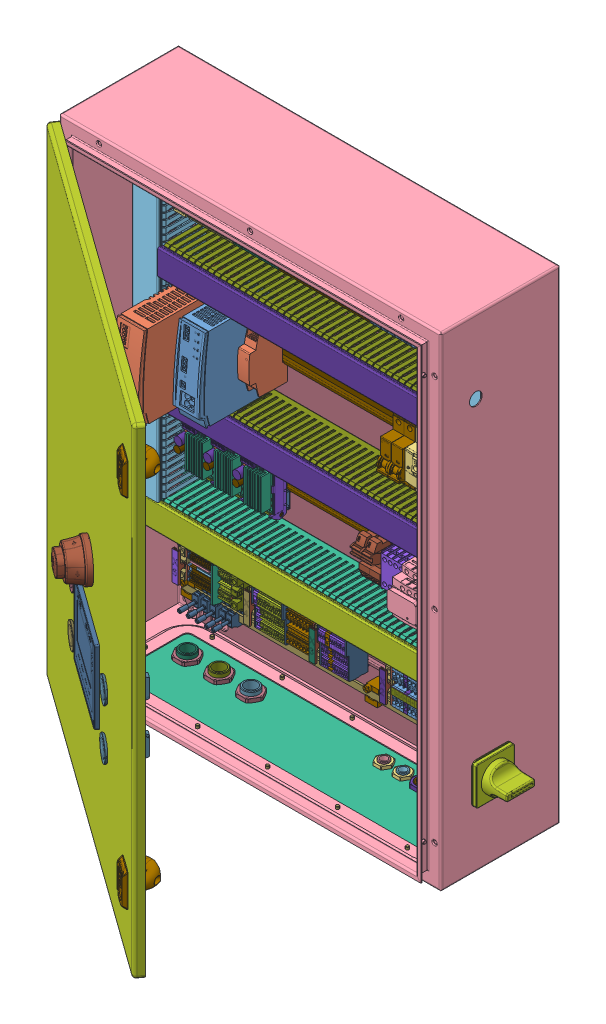
SolidWorks assembly Armoir életrique v46.step, configuration Valor predeterminado. Lengths in mm. (continued)
Components (placement in the parent): (continued)
- Rail bornier complet.step-1: Rail bornier complet.step [Valor predeterminado] at (531.5 121.5 20) x (-1 0 0) z (0 0 1) size (500.55 113.8 62.99) (continued)
  - Barre Raccordement blindage.step-1: Barre Raccordement blindage.step [Valor predeterminado] at (370 -26.6 19.1) x (0 -1 0) z (1 0 0) size (23.95 55.8 120.55) (continued)
    - pxc_3025888_05_AB-SS-M_3D_1.step-1: pxc_3025888_05_AB-SS-M_3D_1.step [Valor predeterminado] at (25.4 25.82 323.5236) x (1 0 0) z (0 -1 0) size (23.95 19.95 23.55) (continued)
      - AB_SS_M-select.step-1: AB_SS_M-select.step [Valor predeterminado] at (-120.3937 -178.9939 26.12) x (-1 0 0) z (0 0 1) size (23.95 19.95 23.55)
    - pxc_3025338_03_SK-5_3D.step-1: pxc_3025338_03_SK-5_3D.step [Valor predeterminado] at (25.4 -45.4 261.5) size (19.5 46.8 9)
      - SK5_select.step-1: SK5_select.step [Valor predeterminado] at (53.9697 30.1229 -268.721) x (0 0 1) z (0 -1 0) size (9 19.5 46.8)
    - pxc_3025338_03_SK-5_3D_1.step-1: pxc_3025338_03_SK-5_3D_1.step [Valor predeterminado] at (25.4 -45.4 280.5) size (19.5 46.8 9)
      - SK5_select.step-1: SK5_select.step [Valor predeterminado] at (53.9697 30.1229 -273.721) x (0 0 1) z (0 -1 0) size (9 19.5 46.8)
    - pxc_3025338_03_SK-5_3D_2.step-1: pxc_3025338_03_SK-5_3D_2.step [Valor predeterminado] at (25.4 -45.4 301.5) size (19.5 46.8 9)
      - SK5_select.step-1: SK5_select.step [Valor predeterminado] at (53.9697 30.1229 -322.721) x (0 0 1) z (0 -1 0) size (9 19.5 46.8)
    - pxc_3025338_03_SK-5_3D_3.step-1: pxc_3025338_03_SK-5_3D_3.step [Valor predeterminado] at (25.4 -45.4 346.5) size (19.5 46.8 9)
      - SK5_select.step-1: SK5_select.step [Valor predeterminado] at (53.9697 30.1229 -382.171) x (0 0 1) z (0 -1 0) size (9 19.5 46.8)
    - pxc_3025338_03_SK-5_3D_4.step-1: pxc_3025338_03_SK-5_3D_4.step [Valor predeterminado] at (25.4 -45.4 360.5) size (19.5 46.8 9)
      - SK5_select.step-1: SK5_select.step [Valor predeterminado] at (53.9697 30.1229 -406.671) x (0 0 1) z (0 -1 0) size (9 19.5 46.8)
    - Barre Raccordement blindage-0.step-1: Barre Raccordement blindage-0.step [Valor predeterminado] at origin size (10 3 120)
  - Barre Raccordement blindage_1.step-1: Barre Raccordement blindage_1.step [Valor predeterminado] at (490 53.6 19.1) x (0 1 0) z (-1 0 0) size (23.95 55.8 500.55)
    - pxc_3025888_05_AB-SS-M_3D_2.step-1: pxc_3025888_05_AB-SS-M_3D_2.step [Valor predeterminado] at (-10.6 12.6 -71.5) x (1 0 0) z (0 -1 0) size (23.95 19.95 23.55)
      - AB_SS_M-select.step-1: AB_SS_M-select.step [Valor predeterminado] at (-84.3937 115.4297 12.9) x (-1 0 0) z (0 0 1) size (23.95 19.95 23.55)
    - pxc_3025888_05_AB-SS-M_3D_3.step-1: pxc_3025888_05_AB-SS-M_3D_3.step [Valor predeterminado] at (-10.6 45.82 -9.4764) x (1 0 0) z (0 -1 0) size (23.95 19.95 23.55)
      - AB_SS_M-select.step-1: AB_SS_M-select.step [Valor predeterminado] at (-84.3937 534.0061 46.12) x (-1 0 0) z (0 0 1) size (23.95 19.95 23.55)
    - pxc_3025338_03_SK-5_3D_5.step-1: pxc_3025338_03_SK-5_3D_5.step [Valor predeterminado] at (-10.6 -25.4 -71.5) size (19.5 46.8 9)
      - SK5_select.step-1: SK5_select.step [Valor predeterminado] at (89.9697 10.1229 22.679) x (0 0 1) z (0 -1 0) size (9 19.5 46.8)
    - pxc_3025338_03_SK-5_3D_6.step-1: pxc_3025338_03_SK-5_3D_6.step [Valor predeterminado] at (-10.6 -25.4 -52.5) size (19.5 46.8 9)
      - SK5_select.step-1: SK5_select.step [Valor predeterminado] at (89.9697 10.1229 17.679) x (0 0 1) z (0 -1 0) size (9 19.5 46.8)
    - pxc_3025338_03_SK-5_3D_7.step-1: pxc_3025338_03_SK-5_3D_7.step [Valor predeterminado] at (-10.6 -25.4 -31.5) size (19.5 46.8 9)
      - SK5_select.step-1: SK5_select.step [Valor predeterminado] at (89.9697 10.1229 10.679) x (0 0 1) z (0 -1 0) size (9 19.5 46.8)
    - pxc_3025888_05_AB-SS-M_3D_4.step-1: pxc_3025888_05_AB-SS-M_3D_4.step [Valor predeterminado] at (-10.6 12.6 -71.5) x (1 0 0) z (0 -1 0) size (23.95 19.95 23.55)
      - AB_SS_M-select.step-1: AB_SS_M-select.step [Valor predeterminado] at (-84.3937 404.8297 12.9) x (-1 0 0) z (0 0 1) size (23.95 19.95 23.55)
    - pxc_3025338_03_SK-5_3D_8.step-1: pxc_3025338_03_SK-5_3D_8.step [Valor predeterminado] at (-10.6 -25.4 -11.5) size (19.5 46.8 9)
      - SK5_select.step-1: SK5_select.step [Valor predeterminado] at (89.9697 10.1229 5.129) x (0 0 1) z (0 -1 0) size (9 19.5 46.8)
    - pxc_3025338_03_SK-5_3D_9.step-1: pxc_3025338_03_SK-5_3D_9.step [Valor predeterminado] at (-10.6 -25.4 3.5) size (19.5 46.8 9)
      - SK5_select.step-1: SK5_select.step [Valor predeterminado] at (89.9697 10.1229 0.629) x (0 0 1) z (0 -1 0) size (9 19.5 46.8)
    - Barre Raccordement blindage_1-1.step-1: Barre Raccordement blindage_1-1.step [Valor predeterminado] at origin size (10 3 500)
- Fond de coffret.step-1: Fond de coffret.step [Valor predeterminado] at (297 -1.5 93.5) x (1 0 0) z (0 -1 0) size (534 149 43)
  - MSV-M25x1.5_16_83602461.step-1: MSV-M25x1.5_16_83602461.step [Valor predeterminado] at (-117 -24.5 1.5) x (0 0 -1) z (1 0 0) size (40 32 35.2)
    - KGM-M25x1,5_83727256.step-1: KGM-M25x1,5_83727256.step [Valor predeterminado] at (1.5 0 0) x (0 1 0) z (0 0 -1) size (32 6 35.2)
    - MSV-M25x1.5_16_83602461-2.step-1: MSV-M25x1.5_16_83602461-2.step [Valor predeterminado] at origin size (40 29.5 29.5)
  - MSV-M25x1.5_16_83602461_1.step-1: MSV-M25x1.5_16_83602461_1.step [Valor predeterminado] at (-217 -24.5 1.5) x (0 0 -1) z (1 0 0) size (40 32 35.2)
    - KGM-M25x1,5_83727256.step-1: KGM-M25x1,5_83727256.step [Valor predeterminado] at (1.5 0 0) x (0 1 0) z (0 0 -1) size (32 6 35.2)
    - MSV-M25x1.5_16_83602461_1-3.step-1: MSV-M25x1.5_16_83602461_1-3.step [Valor predeterminado] at origin size (40 29.5 29.5)
  - MSV-M25x1.5_16_83602461_2.step-1: MSV-M25x1.5_16_83602461_2.step [Valor predeterminado] at (-167 -24.5 1.5) x (0 0 -1) z (1 0 0) size (40 32 35.2)
    - KGM-M25x1,5_83727256.step-1: KGM-M25x1,5_83727256.step [Valor predeterminado] at (1.5 0 0) x (0 1 0) z (0 0 -1) size (32 6 35.2)
    - MSV-M25x1.5_16_83602461_2-4.step-1: MSV-M25x1.5_16_83602461_2-4.step [Valor predeterminado] at origin size (40 29.5 29.5)
  - PFLITSCH bg220 PA.step-1: PFLITSCH bg220 PA.step [Valor predeterminado] at (142 -34.5 1.5) x (1 0 0) z (0 -1 0) size (29 38 26.7)
    - PFLITSCH 1420_220.step-1: PFLITSCH 1420_220.step [Valor predeterminado] at (0 -7.5 0) x (1 0 0) z (0 0 -1) size (29 6 26)
    - PFLITSCH bg220 PA-5.step-1: PFLITSCH bg220 PA-5.step [Valor predeterminado] at origin size (24 38 26.7)
  - PFLITSCH bg220 PA_1.step-1: PFLITSCH bg220 PA_1.step [Valor predeterminado] at (177 -34.5 1.5) x (1 0 0) z (0 -1 0) size (29 38 26.7)
    - PFLITSCH 1420_220.step-1: PFLITSCH 1420_220.step [Valor predeterminado] at (0 -7.5 0) x (1 0 0) z (0 0 -1) size (29 6 26)
    - PFLITSCH bg220 PA_1-6.step-1: PFLITSCH bg220 PA_1-6.step [Valor predeterminado] at origin size (24 38 26.7)
  - PFLITSCH bg220 PA_2.step-1: PFLITSCH bg220 PA_2.step [Valor predeterminado] at (212 -34.5 1.5) x (1 0 0) z (0 -1 0) size (29 38 26.7)
    - PFLITSCH 1420_220.step-1: PFLITSCH 1420_220.step [Valor predeterminado] at (0 -7.5 0) x (1 0 0) z (0 0 -1) size (29 6 26)
    - PFLITSCH bg220 PA_2-7.step-1: PFLITSCH bg220 PA_2-7.step [Valor predeterminado] at origin size (24 38 26.7)
  - PFLITSCH bg216 PA.step-1: PFLITSCH bg216 PA.step [Valor predeterminado] at (82 -34.5 1.5) x (1 0 0) z (0 -1 0) size (25 34 22.2)
    - PFLITSCH 1420_216.step-1: PFLITSCH 1420_216.step [Valor predeterminado] at (0 -6.5 0) x (1 0 0) z (0 0 -1) size (25 5 22)
    - PFLITSCH bg216 PA-8.step-1: PFLITSCH bg216 PA-8.step [Valor predeterminado] at origin size (20.01 34 22.2)
  - PFLITSCH bg216 PA_1.step-1: PFLITSCH bg216 PA_1.step [Valor predeterminado] at (112 -34.5 1.5) x (1 0 0) z (0 -1 0) size (25 34 22.2)
    - PFLITSCH 1420_216.step-1: PFLITSCH 1420_216.step [Valor predeterminado] at (0 -6.5 0) x (1 0 0) z (0 0 -1) size (25 5 22)
    - PFLITSCH bg216 PA_1-9.step-1: PFLITSCH bg216 PA_1-9.step [Valor predeterminado] at origin size (20.01 34 22.2)
  - Fond de coffret-10.step-1: Fond de coffret-10.step [Valor predeterminado] at origin size (534 149 1.5)
- vcf1.step-1: vcf1.step [Valor predeterminado] at (536 118.5 108) x (0 0 -1) z (0 -1 0) size (63 107.61 74.15)
- lp1k0610bd.step-1: lp1k0610bd.step [Valor predeterminado] at (396.4 252.9987 24.0075) size (45 58 56.72)
- 3D_G_I202_XX_18131V.step-1: 3D_G_I202_XX_18131V.step [Valor predeterminado] at (396.7 451.1996 27.5) x (0 1 0) z (0 0 -1) size (89.8 35.2 76.4)
- 6av21232db030ax0.step-1: 6av21232db030ax0.step [Valor predeterminado] at (178.4023 180.9 337.4401) x (0.811697 0 0.584079) z (-0.584079 0 0.811697) size (140 116 41.31)
- xb5as84w3b5.step-1: xb5as84w3b5.step [Valor predeterminado] at (230.9572 364.4 384.251) x (0.811697 0 0.584079) z (0 -1 0) size (59.99 84.54 60.6)
- xb4fa31.step-1: xb4fa31.step [Valor predeterminado] at (125.4304 185.0475 289.825) x (-0.811697 0 -0.584079) z (0 1 0) size (36.41 52.95 53.31)
- xb4fa61.step-1: xb4fa61.step [Valor predeterminado] at (175.444 263.7525 325.8137) x (0.811697 0 0.584079) z (0 -1 0) size (36.41 52.95 53.31)
- XB4FA3351.step-1: XB4FA3351.step [Valor predeterminado] at (354.0173 183.7525 454.3111) x (0.811697 0 0.584079) z (0 -1 0) size (36.41 52.95 53.31)
- XB4FA3351.step-2: XB4FA3351.step [Valor predeterminado] at (304.0037 265.0475 418.3224) x (-0.811697 0 -0.584079) z (0 1 0) size (36.41 52.95 53.31)
